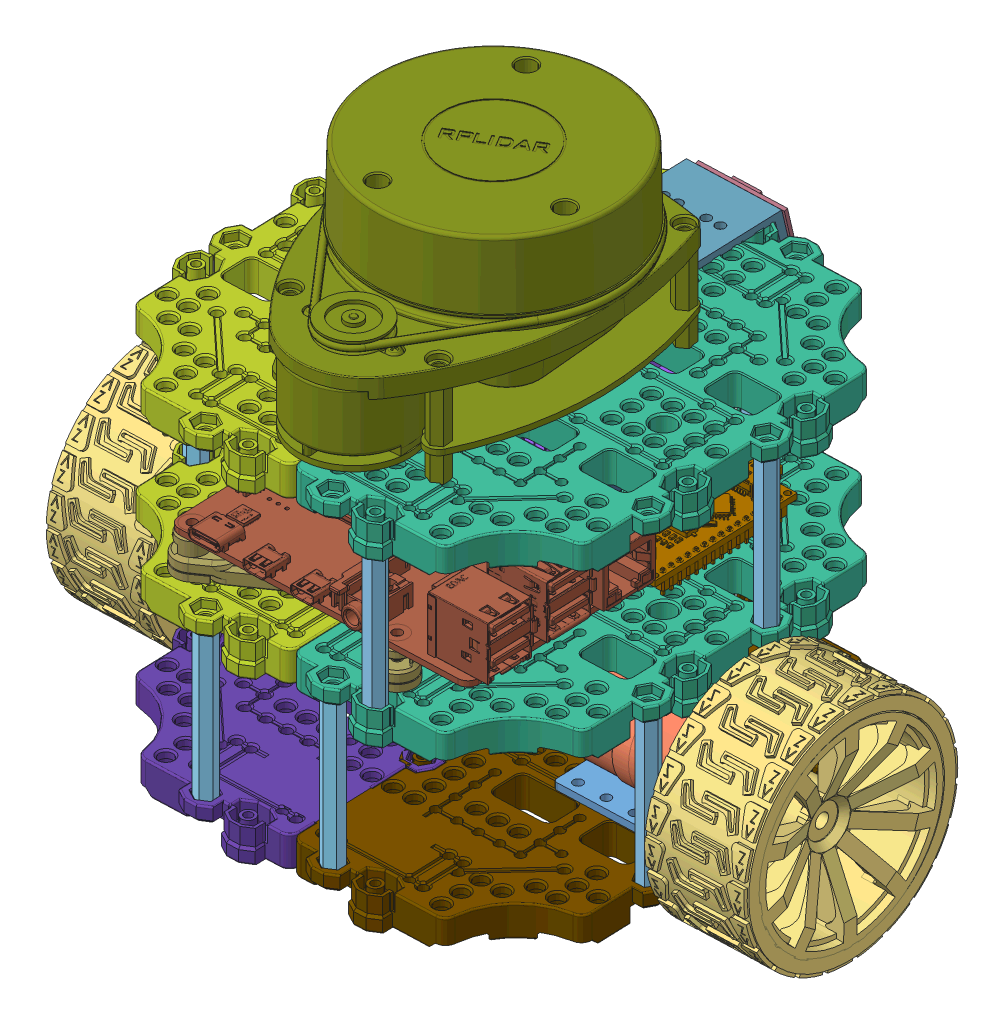
SolidWorks assembly BumperBot, configuration Default. Lengths in mm.
Overall size (264.4 773.19 204.68).
44 component instances, 20 part files, 118 mates.
Components (placement in the parent):
- motor_support-1: motor_support [Default] at (-39.885 107.5277 104.4569) x (-0.035505 0 -0.999369) z (0.999369 0 -0.035505) size (28 29 41)
- motor_support-2: motor_support [Default] at (97.5755 107.5277 99.5732) x (0.035505 0 0.999369) z (-0.999369 0 0.035505) size (28 29 41)
- JGA25-370-1: JGA25-370 [Default] at (52.3299 107.5277 101.1807) x (0.999369 0 -0.035505) z (0 -1 0) size (70.5 25.2 25.2)
- JGA25-370-2: JGA25-370 [Default] at (5.3607 107.5277 102.8494) x (-0.999369 0 0.035505) z (0 -1 0) size (70.5 25.2 25.2)
- wheel-1: wheel [Default] at (-18.4133 64.9311 67.753) x (0.033104 -0.361489 0.931789) z (-0.999369 0 0.035505) size (65.01 65.01 29)
- wheel_motor_adapter-1: wheel_motor_adapter [Default] at (-52.3777 107.532 104.885) x (0.034231 -0.265538 0.963493) z (-0.999369 0 0.035505) size (13.7 12 18.23)
- wheel-2: wheel [Default] at (72.8839 117.7622 45.6451) x (0.0175 0.870089 0.492584) z (0.999369 0 -0.035505) size (65.01 65.01 29)
- wheel_motor_adapter-2: wheel_motor_adapter [Default] at (110.0673 107.5144 99.12) x (0.020529 0.815898 0.577832) z (0.999369 0 -0.035505) size (13.7 12 18.23)
- SUPPORT_HEX_M3_0XL45_FF-1: SUPPORT_HEX_M3_0XL45_FF [Default] at (50.5578 90.0277 37.2033) x (-0.5 0 0.866025) z (-0.866025 0 -0.5) size (5 45 5.77)
- SUPPORT_HEX_M3_0XL45_FF-6: SUPPORT_HEX_M3_0XL45_FF [Default] at (7.1327 90.0277 166.8268) x (0.255141 0 -0.966904) z (0.966904 0 0.255141) size (5 45 5.77)
- waffle_front_plate-3: waffle_front_plate [Default] at (28.8453 139.5277 102.0151) x (0.999369 0 -0.035505) z (0.035505 0 0.999369) size (73.55 9.85 137.55)
- waffle_rear_plate-2: waffle_rear_plate [Default] at (28.8453 139.5277 102.0151) x (-0.999369 0 0.035505) z (-0.035505 0 -0.999369) size (73.55 9.85 137.55)
- SUPPORT_HEX_M3_0XL45_FF-7: SUPPORT_HEX_M3_0XL45_FF [Default] at (2.588 87.5277 38.9075) x (0 0 -1) z (1 0 0) size (5 45 5.77)
- SUPPORT_HEX_M3_0XL45_FF-17: SUPPORT_HEX_M3_0XL45_FF [Default] at (-35.9665 135.0277 80.3025) x (0.866025 0 0.5) z (0.5 0 -0.866025) size (5 45 5.77)
- SUPPORT_HEX_M3_0XL45_FF-18: SUPPORT_HEX_M3_0XL45_FF [Default] at (93.657 135.0277 123.7276) x (0.866025 0 0.5) z (0.5 0 -0.866025) size (5 45 5.77)
- L298N-2: L298N [Default] at (11.4909 149.5277 70.3617) x (0.999369 0 -0.035505) z (0.035505 0 0.999369) size (50 22 50)
- Arduino Nano-2: Arduino Nano [Default] at (42.2606 141.5277 53.4388) x (0.035505 0 0.999369) z (0 1 0) size (44.28 18 13.68)
- board_bracket_small-1: board_bracket_small [Default] at (33.6312 139.5277 47.5214) x (0.998944 0 -0.045937) z (0.045937 0 0.998944) size (37.82 10 10.43)
- board_bracket_small-2: board_bracket_small [Default] at (-10.6494 139.5277 93.2019) x (0.065728 0 0.997838) z (-0.997838 0 0.065728) size (37.82 10 10.43)
- board_bracket_small-3: board_bracket_small [Default] at (35.1962 139.5277 91.5731) x (0.107735 0 0.99418) z (-0.99418 0 0.107735) size (37.82 10 10.43)
- SUPPORT_HEX_M3_0XL45_FF-20: SUPPORT_HEX_M3_0XL45_FF [Default] at (-34.2623 179.8277 128.2723) x (0.530433 0 0.847727) z (0.847727 0 -0.530433) size (5 45 5.77)
- SUPPORT_HEX_M3_0XL45_FF-21: SUPPORT_HEX_M3_0XL45_FF [Default] at (14.5805 182.0277 38.4815) x (-0.999369 0 0.035505) z (0.035505 0 0.999369) size (5 45 5.77)
- SUPPORT_HEX_M3_0XL45_FF-22: SUPPORT_HEX_M3_0XL45_FF [Default] at (-35.5405 179.8277 92.295) x (-0.468936 0 0.883232) z (0.883232 0 0.468936) size (5 45 5.77)
- SUPPORT_HEX_M3_0XL45_FF-23: SUPPORT_HEX_M3_0XL45_FF [Default] at (38.5654 179.8277 37.6293) x (0.035505 0 0.999369) z (0.999369 0 -0.035505) size (5 45 5.77)
- SUPPORT_HEX_M3_0XL45_FF-25: SUPPORT_HEX_M3_0XL45_FF [Default] at (43.11 135.0277 165.5486) x (1 0 0) z (0 0 -1) size (5 45 5.77)
- SUPPORT_HEX_M3_0XL45_FF-26: SUPPORT_HEX_M3_0XL45_FF [Default] at (55.1025 179.8277 165.1226) x (0.883232 0 0.468936) z (0.468936 0 -0.883232) size (5 45 5.77)
- SUPPORT_HEX_M3_0XL45_FF-27: SUPPORT_HEX_M3_0XL45_FF [Default] at (92.3788 182.0277 87.7503) x (0.035505 0 0.999369) z (0.999369 0 -0.035505) size (5 45 5.77)
- Raspberry Pi 4 Model B-3: Raspberry Pi 4 Model B [Default] at (149.9317 65.3277 125.8391) x (0.999369 0 -0.035505) z (0 1 0) size (89.07 58.45 20.84)
- board_bracket-5: board_bracket [Default] at (53.2833 139.5277 156.9085) x (0.727355 0 0.686261) z (-0.686261 0 0.727355) size (37.82 10 10.2)
- board_bracket-6: board_bracket [Default] at (51.5435 139.5277 107.9394) x (-0.255641 0 -0.966772) z (0.966772 0 -0.255641) size (37.82 10 10.2)
- board_bracket-7: board_bracket [Default] at (-4.6801 139.5277 158.9678) x (-0.81984 0 0.572593) z (-0.572593 0 -0.81984) size (37.82 10 10.2)
- board_bracket-8: board_bracket [Default] at (-6.4199 139.5277 109.9987) x (-0.570741 0 -0.82113) z (0.82113 0 -0.570741) size (37.82 10 10.2)
- waffle_rear_plate-3: waffle_rear_plate [Default] at (28.8453 186.5277 102.0151) x (-0.999369 0 0.035505) z (-0.035505 0 -0.999369) size (73.55 9.85 137.55)
- waffle_front_plate-4: waffle_front_plate [Default] at (28.8453 186.8277 102.0151) x (0.999369 0 -0.035505) z (0.035505 0 0.999369) size (73.55 9.85 137.55)
- RPi cam Rev 1.3-1: RPi cam Rev 1.3 [Výchozí] at (26.1362 175.4612 25.7618) x (0.999369 0 -0.035505) z (-0.03451 0.235171 -0.971341) size (25.2 33.1 8.7)
- camera_stand_reversed-1: camera_stand_reversed [Default] at (40.8891 188.5277 60.7879) x (0.035505 0 0.999369) z (-0.999369 0 0.035505) size (34.33 18.42 27)
- MPU_6050-1: MPU_6050 [Default] at (29.2409 176.3277 107.5422) x (1 0 0) z (0 -1 0) size (20.5 16 3)
- RP-lidar-A1-2: RP-lidar-A1 [Default] at (172.287 -533.1647 184.7238) x (0.092466 0 0.995716) z (-0.995716 0 0.092466) size (101.56 53.5 71.81)
- waffle_rear_base_plate-1: waffle_rear_base_plate [Default] at (28.8453 92.5277 102.0151) x (-0.999369 0 0.035505) z (-0.035505 0 -0.999369) size (73.55 9.85 137.55)
- waffle_front_base_plate-1: waffle_front_base_plate [Default] at (28.8453 92.5277 102.0151) x (0.999369 0 -0.035505) z (0.035505 0 0.999369) size (73.55 9.85 137.55)
- waffle_caster_support-4: waffle_caster_support [Default] at (30.5335 86.0277 149.5351) x (-0.999369 0 0.035505) z (0.035505 0 0.999369) size (30 8.25 18.16)
- waffle_caster_support-5: waffle_caster_support [Default] at (27.157 86.0277 54.495) x (-0.999369 0 0.035505) z (0.035505 0 0.999369) size (30 8.25 18.16)
- waffle_caster_ball-4: waffle_caster_ball [Default] at (30.5335 82.1652 149.5351) size (9.53 9.53 9.53)
- waffle_caster_ball-5: waffle_caster_ball [Default] at (27.157 82.1652 54.495) size (9.53 9.53 9.53)
Mates (geometry in assembly coordinates):
- Coincident21: coincident anti-aligned: plane of motor_support-2 through (95.5768 107.5277 99.6442) normal (-0.999369 0 0.035505); plane of JGA25-370-1 through (96.0206 107.5277 112.1363) normal (0.999369 0 -0.035505)
- Concentric7: concentric aligned: circle of motor_support-2; circle of JGA25-370-1
- Concentric8: concentric aligned: cylinder of motor_support-2 through (95.275 107.5277 91.1496) axis (0.999369 0 -0.035505) radius 1.25; cylinder of JGA25-370-1 through (90.2781 107.5277 91.3271) axis (0.999369 0 -0.035505) radius 1.25
- Coincident22: coincident anti-aligned: plane of motor_support-1 through (-37.8863 107.5277 104.3859) normal (0.999369 0 -0.035505); plane of JGA25-370-2 through (-38.3301 107.5277 91.8938) normal (-0.999369 0 0.035505)
- Concentric9: concentric aligned: circle of motor_support-1; circle of JGA25-370-2
- Concentric10: concentric anti-aligned: circle of motor_support-1; circle of JGA25-370-2
- Coincident24: coincident anti-aligned: plane of wheel-1 through (-58.4359 114.2363 103.3532) normal (-0.009428 -0.964101 -0.26537); plane of wheel_motor_adapter-1 through (-58.1987 112.3966 110.0284) normal (0.009428 0.964101 0.26537)
- Coincident25: coincident anti-aligned: plane of wheel-1 through (-58.1367 105.6921 111.7739) normal (-0.024931 0.712013 -0.701724); plane of wheel_motor_adapter-1 through (-58.3119 100.8274 106.844) normal (0.024931 -0.712013 0.701724)
- Coincident26: coincident anti-aligned: plane of wheel-1 through (-58.3739 107.5318 105.0986) normal (0.999369 0 -0.035505); plane of wheel_motor_adapter-1 through (-58.3739 107.532 105.0981) normal (-0.999369 0 0.035505)
- Concentric11: concentric aligned: cylinder of JGA25-370-2 through (-50.3784 107.5277 104.8297) axis (0.999369 0 -0.035505) radius 1.95; cylinder of wheel_motor_adapter-1 through (-52.3771 107.5277 104.9007) axis (0.999369 0 -0.035505) radius 3
- Coincident30: coincident anti-aligned: plane of wheel-2 through (116.1662 101.2193 101.7979) normal (-0.028969 0.578196 -0.815383); plane of wheel_motor_adapter-2 through (116.3085 106.872 105.8012) normal (0.028969 -0.578196 0.815383)
- Coincident31: coincident anti-aligned: plane of wheel-2 through (116.3085 106.872 105.8012) normal (-0.032263 -0.41749 -0.908108); plane of wheel_motor_adapter-2 through (116.2058 113.1675 102.9106) normal (0.032263 0.41749 0.908108)
- Coincident32: coincident anti-aligned: plane of wheel-2 through (116.0635 107.5148 98.9073) normal (-0.999369 0 0.035505); plane of wheel_motor_adapter-2 through (116.0635 107.5144 98.907) normal (0.999369 0 -0.035505)
- Concentric16: concentric aligned: cylinder of JGA25-370-1 through (108.0689 107.5277 99.2004) axis (-0.999369 0 0.035505) radius 1.95; cylinder of wheel_motor_adapter-2 through (110.0676 107.5277 99.1294) axis (-0.999369 0 0.035505) radius 3
- Coincident33: coincident anti-aligned: plane of JGA25-370-1 through (98.0752 107.5277 99.5555) normal (0.999369 0 -0.035505); plane of wheel_motor_adapter-2 through (98.0749 107.5144 99.5461) normal (-0.999369 0 0.035505)
- Coincident34: coincident anti-aligned: plane of JGA25-370-2 through (-40.3847 107.5277 104.4746) normal (-0.999369 0 0.035505); plane of wheel_motor_adapter-1 through (-40.3852 107.532 104.459) normal (0.999369 0 -0.035505)
- Coincident72: coincident anti-aligned: plane of SUPPORT_HEX_M3_0XL45_FF-1 through (50.5578 135.0277 37.2033) normal (0 1 0); plane of waffle_front_plate-3 through (28.8453 135.0277 102.0151) normal (0 -1 0)
- Concentric28: concentric anti-aligned: cylinder of SUPPORT_HEX_M3_0XL45_FF-1 through (50.5578 123.739 37.2033) axis (0 -1 0) radius 1.25; cylinder of waffle_front_plate-3 through (50.5578 129.1327 37.2033) axis (0 1 0) radius 1.6
- Concentric30: concentric anti-aligned: cylinder of SUPPORT_HEX_M3_0XL45_FF-6 through (7.1327 123.739 166.8268) axis (0 -1 0) radius 1.25; cylinder of waffle_rear_plate-2 through (7.1327 129.1327 166.8268) axis (0 1 0) radius 1.6
- Coincident74: coincident anti-aligned: plane of SUPPORT_HEX_M3_0XL45_FF-6 through (7.1327 135.0277 166.8268) normal (0 1 0); plane of waffle_rear_plate-2 through (28.8453 135.0277 102.0151) normal (0 -1 0)
- Concentric33: concentric aligned: circle of waffle_rear_plate-2; circle of SUPPORT_HEX_M3_0XL45_FF-7
- Parallel33: parallel aligned: plane of waffle_rear_plate-2 through (14.411 137.2777 33.711) normal (-0.035505 0 -0.999369); plane of L298N-2 through (-14.381 150.5277 46.2651) normal (-0.035505 0 -0.999369)
- Parallel34: parallel anti-aligned: plane of waffle_front_plate-3 through (28.8453 139.5277 102.0151) normal (0 1 0); plane of L298N-2 through (11.4909 149.5277 70.3617) normal (0 -1 0)
- Parallel35: parallel aligned: plane of waffle_front_plate-3 through (90.5326 139.5277 35.7831) normal (-0.035505 0 -0.999369); plane of Arduino Nano-2 through (70.9901 145.6677 57.4663) normal (-0.035505 0 -0.999369)
- Parallel36: parallel anti-aligned: plane of waffle_front_plate-3 through (28.8453 139.5277 102.0151) normal (0 1 0); plane of Arduino Nano-2 through (54.5159 144.0677 61.864) normal (0 -1 0)
- Concentric72: concentric aligned: cylinder of L298N-2 through (33.6312 149.5277 47.5214) axis (0 1 0) radius 1.5; circle of board_bracket_small-1
- Coincident123: coincident anti-aligned: plane of L298N-2 through (11.4909 149.5277 70.3617) normal (0 -1 0); plane of board_bracket_small-1 through (33.6312 149.5277 47.5214) normal (0 1 0)
- Coincident124: coincident anti-aligned: plane of waffle_rear_plate-2 through (28.8453 139.5277 102.0151) normal (0 1 0); plane of board_bracket_small-1 through (5.9412 139.5277 48.7947) normal (0 -1 0)
- Concentric73: concentric anti-aligned: cylinder of waffle_rear_plate-2 through (5.9412 139.5277 48.7947) axis (0 -1 0) radius 2.5; cylinder of board_bracket_small-1 through (5.9412 126.4917 48.7947) axis (0 1 0) radius 5
- Lock5: lock: unknown of waffle_front_plate-3; unknown of board_bracket_small-1
- Concentric75: concentric aligned: circle of L298N-2; cylinder of board_bracket_small-2 through (-10.6494 149.5277 93.2019) axis (0 1 0) radius 1
- Coincident125: coincident anti-aligned: plane of L298N-2 through (11.4909 149.5277 70.3617) normal (0 -1 0); plane of board_bracket_small-2 through (-10.6494 149.5277 93.2019) normal (0 1 0)
- Lock6: lock: unknown of waffle_rear_plate-2; unknown of board_bracket_small-2
- Concentric78: concentric aligned: cylinder of L298N-2 through (35.1962 149.5277 91.5731) axis (0 1 0) radius 1.5; cylinder of board_bracket_small-3 through (35.1962 149.5277 91.5731) axis (0 1 0) radius 1
- Coincident126: coincident anti-aligned: plane of L298N-2 through (11.4909 149.5277 70.3617) normal (0 -1 0); plane of board_bracket_small-3 through (35.1962 149.5277 91.5731) normal (0 1 0)
- Lock7: lock: unknown of waffle_front_plate-3; unknown of board_bracket_small-3
- Concentric81: concentric aligned: circle of waffle_rear_plate-2; cylinder of SUPPORT_HEX_M3_0XL45_FF-20 through (-34.2623 146.1163 128.2723) axis (0 1 0) radius 1.25
- Coincident129: coincident anti-aligned: plane of waffle_rear_plate-2 through (28.8453 134.8277 102.0151) normal (0 1 0); plane of SUPPORT_HEX_M3_0XL45_FF-20 through (-34.2623 134.8277 128.2723) normal (0 -1 0)
- Parallel44: parallel aligned: plane of waffle_rear_plate-2 through (-38.4889 139.5277 126.8502) normal (-0.999369 0 0.035505); plane of SUPPORT_HEX_M3_0XL45_FF-20 through (-36.7094 179.8277 129.8035) normal (-0.999369 0 0.035505)
- Concentric82: concentric aligned: cylinder of waffle_rear_plate-2 through (14.5805 129.1327 38.4815) axis (0 1 0) radius 1.6; cylinder of SUPPORT_HEX_M3_0XL45_FF-21 through (14.5805 148.3163 38.4815) axis (0 1 0) radius 1.25
- Coincident131: coincident anti-aligned: plane of waffle_rear_plate-2 through (28.8453 137.0277 102.0151) normal (0 1 0); plane of SUPPORT_HEX_M3_0XL45_FF-21 through (14.5805 137.0277 38.4815) normal (0 -1 0)
- Concentric83: concentric anti-aligned: cylinder of waffle_rear_plate-2 through (-35.5405 139.5277 92.295) axis (0 1 0) radius 1.2; circle of SUPPORT_HEX_M3_0XL45_FF-22
- Coincident133: coincident anti-aligned: plane of waffle_rear_plate-2 through (28.8453 134.8277 102.0151) normal (0 1 0); plane of SUPPORT_HEX_M3_0XL45_FF-22 through (-35.5405 134.8277 92.295) normal (0 -1 0)
- Parallel46: parallel aligned: plane of waffle_rear_plate-2 through (-39.7671 139.5277 90.8729) normal (-0.999369 0 0.035505); plane of SUPPORT_HEX_M3_0XL45_FF-22 through (-37.9876 179.8277 93.8262) normal (-0.999369 0 0.035505)
- Concentric84: concentric aligned: cylinder of waffle_front_plate-3 through (38.5654 139.5277 37.6293) axis (0 1 0) radius 1.2; cylinder of SUPPORT_HEX_M3_0XL45_FF-23 through (38.5654 146.1163 37.6293) axis (0 1 0) radius 1.25
- Coincident135: coincident anti-aligned: plane of waffle_front_plate-3 through (28.8453 134.8277 102.0151) normal (0 1 0); plane of SUPPORT_HEX_M3_0XL45_FF-23 through (38.5654 134.8277 37.6293) normal (0 -1 0)
- Parallel47: parallel aligned: plane of waffle_front_plate-3 through (39.9875 139.5277 33.4027) normal (-0.035505 0 -0.999369); plane of SUPPORT_HEX_M3_0XL45_FF-23 through (37.0341 179.8277 35.1822) normal (-0.035505 0 -0.999369)
- Concentric87: concentric aligned: cylinder of waffle_front_plate-3 through (55.1025 139.5277 165.1226) axis (0 1 0) radius 1.2; cylinder of SUPPORT_HEX_M3_0XL45_FF-26 through (55.1025 146.1163 165.1226) axis (0 1 0) radius 1.25
- Coincident141: coincident anti-aligned: plane of waffle_front_plate-3 through (28.8453 134.8277 102.0151) normal (0 1 0); plane of SUPPORT_HEX_M3_0XL45_FF-26 through (55.1025 134.8277 165.1226) normal (0 -1 0)
- Parallel50: parallel aligned: plane of waffle_front_plate-3 through (53.6804 139.5277 169.3492) normal (0.035505 0 0.999369); plane of SUPPORT_HEX_M3_0XL45_FF-26 through (56.6337 179.8277 167.5697) normal (0.035505 0 0.999369)
- Concentric88: concentric aligned: circle of waffle_front_plate-3; cylinder of SUPPORT_HEX_M3_0XL45_FF-27 through (92.3788 148.3163 87.7503) axis (0 1 0) radius 1.25
- Coincident143: coincident anti-aligned: plane of waffle_front_plate-3 through (28.8453 137.0277 102.0151) normal (0 1 0); plane of SUPPORT_HEX_M3_0XL45_FF-27 through (92.3788 137.0277 87.7503) normal (0 -1 0)
- Parallel51: parallel aligned: plane of waffle_front_plate-3 through (95.4413 139.5277 92.6446) normal (0.883232 0 0.468936); plane of SUPPORT_HEX_M3_0XL45_FF-27 through (95.2638 182.0277 87.6478) normal (0.883232 0 0.468936)
- Parallel52: parallel anti-aligned: plane of waffle_rear_plate-2 through (28.8453 139.5277 102.0151) normal (0 1 0); plane of Raspberry Pi 4 Model B-3 through (-5.1621 149.5277 159.4852) normal (0 -1 0)
- Parallel53: parallel aligned: plane of waffle_front_plate-3 through (31.1176 139.5277 165.9747) normal (0.035505 0 0.999369); plane of Raspberry Pi 4 Model B-3 through (-5.0556 151.1277 162.4833) normal (0.035505 0 0.999369)
- Parallel54: parallel aligned: plane of waffle_front_plate-3 through (95.0773 139.5277 163.7024) normal (0.999369 0 -0.035505); plane of Raspberry Pi 4 Model B-3 through (76.7862 151.1277 156.5738) normal (0.999369 0 -0.035505)
- Coincident148: coincident aligned: plane of waffle_front_plate-3 through (54.933 137.2777 160.3521) normal (0.035505 0 0.999369); plane of Raspberry Pi 4 Model B-3 through (-5.0556 151.1277 162.4833) normal (0.035505 0 0.999369)
- Concentric90: concentric anti-aligned: cylinder of Raspberry Pi 4 Model B-3 through (53.2833 149.4277 156.9085) axis (0 1 0) radius 1.35; cylinder of board_bracket-5 through (53.2833 150.5277 156.9085) axis (0 -1 0) radius 2
- Coincident149: coincident anti-aligned: plane of Raspberry Pi 4 Model B-3 through (-5.1621 149.5277 159.4852) normal (0 -1 0); plane of board_bracket-5 through (46.2152 149.5277 157.1139) normal (0 1 0)
- Coincident150: coincident anti-aligned: plane of waffle_front_plate-3 through (28.8453 139.5277 102.0151) normal (0 1 0); plane of board_bracket-5 through (47.6699 139.5277 158.4865) normal (0 -1 0)
- Concentric91: concentric aligned: cylinder of waffle_front_plate-3 through (33.1216 138.7277 137.8858) axis (0 1 0) radius 2; cylinder of board_bracket-5 through (33.1216 126.4917 137.8858) axis (0 1 0) radius 5
- Concentric92: concentric anti-aligned: cylinder of Raspberry Pi 4 Model B-3 through (51.5435 149.4277 107.9394) axis (0 1 0) radius 1.35; cylinder of board_bracket-6 through (51.5435 150.5277 107.9394) axis (0 -1 0) radius 2
- Coincident151: coincident anti-aligned: plane of Raspberry Pi 4 Model B-3 through (-5.1621 149.5277 159.4852) normal (0 -1 0); plane of board_bracket-6 through (57.6556 149.5277 111.495) normal (0 1 0)
- Lock8: lock: unknown of waffle_front_plate-3; unknown of board_bracket-6
- Concentric94: concentric anti-aligned: cylinder of Raspberry Pi 4 Model B-3 through (-4.6801 149.4277 158.9678) axis (0 1 0) radius 1.35; cylinder of board_bracket-7 through (-4.6801 150.5277 158.9678) axis (0 -1 0) radius 2
- Coincident152: coincident anti-aligned: plane of Raspberry Pi 4 Model B-3 through (-5.1621 149.5277 159.4852) normal (0 -1 0); plane of board_bracket-7 through (-3.4439 149.5277 152.0056) normal (0 1 0)
- Lock9: lock: unknown of waffle_rear_plate-2; unknown of board_bracket-7
- Concentric96: concentric anti-aligned: cylinder of Raspberry Pi 4 Model B-3 through (-6.4199 149.4277 109.9987) axis (0 1 0) radius 1.3; cylinder of board_bracket-8 through (-6.4199 150.5277 109.9987) axis (0 -1 0) radius 2
- Coincident153: coincident anti-aligned: plane of Raspberry Pi 4 Model B-3 through (-5.1621 149.5277 159.4852) normal (0 -1 0); plane of board_bracket-8 through (0.5395 149.5277 111.2506) normal (0 1 0)
- Lock10: lock: unknown of waffle_rear_plate-2; unknown of board_bracket-8
- Parallel58: parallel anti-aligned: plane of waffle_rear_plate-2 through (17.3213 139.5277 36.7665) normal (-0.468936 0 0.883232); plane of SUPPORT_HEX_M3_0XL45_FF-21 through (14.478 182.0277 35.5965) normal (0.468936 0 -0.883232)
- Concentric98: concentric aligned: cylinder of SUPPORT_HEX_M3_0XL45_FF-21 through (14.5805 170.739 38.4815) axis (0 1 0) radius 1.25; cylinder of waffle_rear_plate-3 through (14.5805 176.1327 38.4815) axis (0 1 0) radius 1.6
- Coincident156: coincident anti-aligned: plane of SUPPORT_HEX_M3_0XL45_FF-21 through (14.5805 182.0277 38.4815) normal (0 1 0); plane of waffle_rear_plate-3 through (28.8453 182.0277 102.0151) normal (0 -1 0)
- Concentric99: concentric aligned: cylinder of SUPPORT_HEX_M3_0XL45_FF-20 through (-34.2623 168.539 128.2723) axis (0 1 0) radius 1.25; cylinder of waffle_rear_plate-3 through (-34.2623 186.5277 128.2723) axis (0 1 0) radius 1.2
- Concentric100: concentric aligned: cylinder of SUPPORT_HEX_M3_0XL45_FF-23 through (38.5654 168.539 37.6293) axis (0 1 0) radius 1.25; cylinder of waffle_front_plate-4 through (38.5654 176.4327 37.6293) axis (0 1 0) radius 1.6
- Coincident157: coincident anti-aligned: plane of SUPPORT_HEX_M3_0XL45_FF-23 through (38.5654 179.8277 37.6293) normal (0 1 0); plane of waffle_front_plate-4 through (28.8453 179.8277 102.0151) normal (0 -1 0)
- Concentric101: concentric aligned: cylinder of SUPPORT_HEX_M3_0XL45_FF-26 through (55.1025 168.539 165.1226) axis (0 1 0) radius 1.25; cylinder of waffle_front_plate-4 through (55.1025 186.8277 165.1226) axis (0 1 0) radius 1.2
- Concentric114: concentric aligned: cylinder of waffle_front_plate-4 through (34.7809 176.4327 43.7676) axis (0 1 0) radius 1.35; cylinder of camera_stand_reversed-1 through (34.7809 168.5277 43.7676) axis (0 1 0) radius 1.35
- Concentric115: concentric anti-aligned: cylinder of waffle_rear_plate-3 through (19.2171 176.1327 56.3281) axis (0 -1 0) radius 1.35; cylinder of camera_stand_reversed-1 through (19.2171 168.5277 56.3281) axis (0 1 0) radius 1.35
- Coincident171: coincident anti-aligned: plane of waffle_rear_plate-3 through (28.8453 186.5277 102.0151) normal (0 1 0); plane of camera_stand_reversed-1 through (13.9061 186.5277 61.7466) normal (0 -1 0)
- Coincident172: coincident anti-aligned: plane of RPi cam Rev 1.3-1 through (26.2155 174.9203 27.9959) normal (0.03451 -0.235171 0.971341); plane of camera_stand_reversed-1 through (12.6871 170.6246 27.4365) normal (-0.03451 0.235171 -0.971341)
- Concentric116: concentric aligned: cylinder of RPi cam Rev 1.3-1 through (36.7492 185.14 28.7575) axis (-0.03451 0.235171 -0.971341) radius 1.05; cylinder of camera_stand_reversed-1 through (37.4843 180.1308 49.4471) axis (-0.03451 0.235171 -0.971341) radius 1
- Concentric117: concentric aligned: cylinder of RPi cam Rev 1.3-1 through (15.6597 173.1849 26.6124) axis (-0.03451 0.235171 -0.971341) radius 1.05; cylinder of camera_stand_reversed-1 through (16.3948 168.1758 47.3019) axis (-0.03451 0.235171 -0.971341) radius 1
- Coincident173: coincident anti-aligned: plane of waffle_front_plate-4 through (28.8453 177.8277 102.0151) normal (0 -1 0); plane of MPU_6050-1 through (29.2409 177.8277 107.5422) normal (0 1 0)
- Concentric119: concentric aligned: circle of waffle_rear_plate-3; cylinder of MPU_6050-1 through (21.2409 176.3277 113.2922) axis (0 1 0) radius 1.5
- Coincident174: coincident anti-aligned: plane of waffle_rear_plate-3 through (28.8453 186.5277 102.0151) normal (0 1 0); plane of RP-lidar-A1-2 through (55.3637 186.5277 146.8196) normal (0 -1 0)
- Concentric121: concentric anti-aligned: cylinder of waffle_rear_plate-3 through (15.535 186.5277 150.5182) axis (0 -1 0) radius 2.5; cylinder of RP-lidar-A1-2 through (15.535 203.6277 150.5182) axis (0 1 0) radius 1
- Lock11: lock: unknown of waffle_front_plate-4; unknown of RP-lidar-A1-2
- Concentric122: concentric anti-aligned: cylinder of waffle_front_plate-3 through (43.11 129.1327 165.5486) axis (0 1 0) radius 1.6; circle of SUPPORT_HEX_M3_0XL45_FF-25
- Concentric124: concentric anti-aligned: cylinder of SUPPORT_HEX_M3_0XL45_FF-6 through (7.1327 101.3163 166.8268) axis (0 -1 0) radius 1.25; cylinder of waffle_rear_base_plate-1 through (7.1327 82.1327 166.8268) axis (0 1 0) radius 1.6
- Coincident178: coincident anti-aligned: plane of SUPPORT_HEX_M3_0XL45_FF-6 through (7.1327 90.0277 166.8268) normal (0 -1 0); plane of waffle_rear_base_plate-1 through (28.8453 90.0277 102.0151) normal (0 1 0)
- Concentric125: concentric anti-aligned: cylinder of SUPPORT_HEX_M3_0XL45_FF-7 through (2.588 98.8163 38.9075) axis (0 -1 0) radius 1.25; cylinder of waffle_rear_base_plate-1 through (2.588 92.5277 38.9075) axis (0 1 0) radius 1.2
- Coincident179: coincident anti-aligned: plane of motor_support-1 through (-38.3833 92.5277 90.3947) normal (0 -1 0); plane of waffle_rear_base_plate-1 through (28.8453 92.5277 102.0151) normal (0 1 0)
- Coincident180: coincident anti-aligned: circle of motor_support-1; cylinder of waffle_rear_base_plate-1 through (-2.744 83.5277 114.1443) axis (0 -1 0) radius 1.35
- Concentric126: concentric anti-aligned: cylinder of motor_support-1 through (-27.51 77.5277 93.0103) axis (0 1 0) radius 1.35; cylinder of waffle_rear_base_plate-1 through (-27.51 83.5277 93.0103) axis (0 -1 0) radius 1.35
- Coincident181: coincident anti-aligned: plane of waffle_front_plate-3 through (28.8453 135.0277 102.0151) normal (0 -1 0); plane of SUPPORT_HEX_M3_0XL45_FF-25 through (43.11 135.0277 165.5486) normal (0 1 0)
- Coincident182: coincident anti-aligned: plane of waffle_front_plate-3 through (28.8453 135.0277 102.0151) normal (0 -1 0); plane of SUPPORT_HEX_M3_0XL45_FF-18 through (93.657 135.0277 123.7276) normal (0 1 0)
- Coincident184: coincident anti-aligned: plane of waffle_rear_plate-2 through (28.8453 132.5277 102.0151) normal (0 -1 0); plane of SUPPORT_HEX_M3_0XL45_FF-7 through (2.588 132.5277 38.9075) normal (0 1 0)
- Coincident185: coincident anti-aligned: plane of waffle_rear_plate-2 through (28.8453 135.0277 102.0151) normal (0 -1 0); plane of SUPPORT_HEX_M3_0XL45_FF-17 through (-35.9665 135.0277 80.3025) normal (0 1 0)
- Concentric127: concentric anti-aligned: cylinder of waffle_front_plate-3 through (93.657 129.1327 123.7276) axis (0 1 0) radius 1.6; circle of SUPPORT_HEX_M3_0XL45_FF-18
- Concentric128: concentric anti-aligned: circle of waffle_rear_plate-2; cylinder of SUPPORT_HEX_M3_0XL45_FF-17 through (-35.9665 123.739 80.3025) axis (0 1 0) radius 1.25
- Concentric129: concentric aligned: cylinder of SUPPORT_HEX_M3_0XL45_FF-17 through (-35.9665 123.739 80.3025) axis (0 1 0) radius 1.25; cylinder of waffle_rear_base_plate-1 through (-35.9665 82.1327 80.3025) axis (0 1 0) radius 1.6
- Coincident186: coincident anti-aligned: plane of waffle_front_plate-3 through (28.8453 139.5277 102.0151) normal (0 1 0); plane of Arduino Nano-2 through (54.5159 139.5277 61.864) normal (0 -1 0)
- Coincident187: coincident aligned: plane of waffle_front_plate-3 through (71.6656 139.5277 76.4786) normal (0.999369 0 -0.035505); plane of Arduino Nano-2 through (70.9901 145.6677 57.4663) normal (0.999369 0 -0.035505)
- Concentric130: concentric anti-aligned: circle of waffle_rear_base_plate-1; cylinder of waffle_front_base_plate-1 through (29.6974 92.5277 125.9999) axis (0 1 0) radius 1.2
- Concentric131: concentric aligned: cylinder of waffle_rear_base_plate-1 through (27.9931 92.5277 78.0302) axis (0 1 0) radius 1.2; cylinder of waffle_front_base_plate-1 through (27.9931 82.1327 78.0302) axis (0 1 0) radius 1.6
- Coincident189: coincident aligned: plane of waffle_rear_base_plate-1 through (18.7541 87.5277 155.9574) normal (0 -1 0); plane of waffle_front_base_plate-1 through (42.739 87.5277 155.1052) normal (0 -1 0)
- Coincident190: coincident anti-aligned: plane of motor_support-2 through (96.0739 92.5277 113.6354) normal (0 -1 0); plane of waffle_front_base_plate-1 through (28.8453 92.5277 102.0151) normal (0 1 0)
- Concentric132: concentric anti-aligned: cylinder of motor_support-2 through (61.2156 77.5277 111.8719) axis (0 1 0) radius 1.35; cylinder of waffle_front_base_plate-1 through (61.2156 83.5277 111.8719) axis (0 -1 0) radius 1.35
- Concentric133: concentric anti-aligned: cylinder of motor_support-2 through (84.4194 77.5277 89.0337) axis (0 1 0) radius 1.35; cylinder of waffle_front_base_plate-1 through (84.4194 83.5277 89.0337) axis (0 -1 0) radius 1.35
- Coincident191: coincident anti-aligned: plane of waffle_front_base_plate-1 through (42.739 87.5277 155.1052) normal (0 -1 0); plane of waffle_caster_support-4 through (30.5335 87.5277 149.5351) normal (0 1 0)
- Concentric134: concentric anti-aligned: cylinder of waffle_front_base_plate-1 through (42.3129 91.5277 143.1128) axis (0 -1 0) radius 2; cylinder of waffle_caster_support-4 through (42.3129 86.7277 143.1128) axis (0 1 0) radius 2.01
- Coincident192: coincident anti-aligned: plane of waffle_rear_base_plate-1 through (14.9515 87.5277 48.9249) normal (0 -1 0); plane of waffle_caster_support-5 through (27.157 87.5277 54.495) normal (0 1 0)
- Concentric140: concentric anti-aligned: cylinder of waffle_rear_base_plate-1 through (15.3776 91.5277 60.9173) axis (0 -1 0) radius 2; cylinder of waffle_caster_support-5 through (15.3776 86.7277 60.9173) axis (0 1 0) radius 2.01
- Concentric141: concentric anti-aligned: cylinder of waffle_front_base_plate-1 through (38.9364 91.5277 48.0728) axis (0 -1 0) radius 2; cylinder of waffle_caster_support-5 through (38.9364 86.7277 48.0728) axis (0 1 0) radius 2.01
- Concentric144: concentric anti-aligned: cylinder of waffle_front_base_plate-1 through (42.739 91.5277 155.1052) axis (0 -1 0) radius 2; cylinder of waffle_caster_support-4 through (42.739 86.7277 155.1052) axis (0 1 0) radius 2.01
- Concentric145: concentric: sphere of waffle_caster_support-4; unknown of waffle_caster_ball-4
- Concentric146: concentric: unknown of waffle_caster_support-5; unknown of waffle_caster_ball-5
